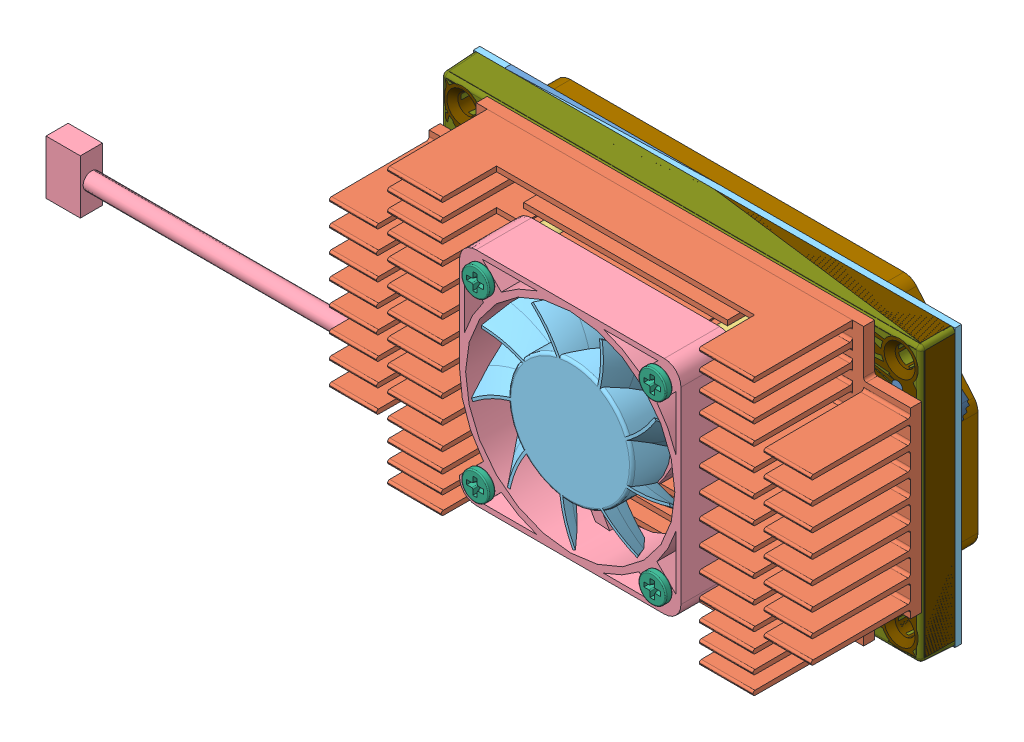
SolidWorks assembly JETSON-NEW_ASM, configuration Default. Lengths in mm.
Overall size (144.7 50.01 33.46).
1881 component instances, 227 part files, 0 mates.
Components (placement in the parent):
- 244-82180-1000-A01-07-31-15_ASM-1: 244-82180-1000-A01-07-31-15_ASM [Default] at origin size (87 50 8.3)
  - 142-82180-1000-A01-07-31-15-1: 142-82180-1000-A01-07-31-15 [Default] at origin size (87 50 1.16)
  - 316-0254-000_2-1: 316-0254-000_2 [Default] at (68.553 22.011 0) x (1 0 0) z (0 0 -1) size (3.51 3.51 0.8)
  - 316-0254-000_2-2: 316-0254-000_2 [Default] at (58.553 17.504 0) x (0 1 0) z (0 0 -1) size (3.51 3.51 0.8)
  - 032-0637-000_1-1: 032-0637-000_1 [Default] at (72.8 30 1.164) size (3.82 1.6 1.8)
  - 032-0637-000_1-2: 032-0637-000_1 [Default] at (72.8 32.06 1.164) size (3.82 1.6 1.8)
  - 032-0628-000_1-1: 032-0628-000_1 [Default] at (53.83 22.43 0) x (0 -1 0) z (0 0 -1) size (3.82 1.6 1.8)
  - 032-0628-000_1-2: 032-0628-000_1 [Default] at (55.94 22.44 0) x (0 -1 0) z (0 0 -1) size (3.82 1.6 1.8)
  - 032-0628-000_1-3: 032-0628-000_1 [Default] at (11.83 6.48 1.164) x (0 1 0) z (0 0 1) size (3.82 1.6 1.8)
  - 032-0628-000_1-4: 032-0628-000_1 [Default] at (13.96 6.5 1.164) x (0 1 0) z (0 0 1) size (3.82 1.6 1.8)
  - RES_04_SMD_015X032_0750-1: RES_04_SMD_015X032_0750 [Default] at (12.96 1.05 1.164) x (0 -1 0) z (0 0 1) size (2.76 3.51 0.75)
  - QFN048Q_P040_0060_T045X04_1000-1: QFN048Q_P040_0060_T045X04_1000 [Default] at (74.15 8.8 1.164) x (0 1 0) z (0 0 1) size (6 6 1)
  - 320-1075-000_1-1: 320-1075-000_1 [Default] at (5.85 26.7 1.164) x (-1 0 0) z (0 0 1) size (4.5 0.8 0.86)
  - 320-1075-000_1-2: 320-1075-000_1 [Default] at (16.1 38.75 1.164) size (4.5 0.8 0.86)
  - 320-1075-000_1-3: 320-1075-000_1 [Default] at (20.1 32.7 1.164) x (0 1 0) z (0 0 1) size (4.5 0.8 0.86)
  - 320-1075-000_1-4: 320-1075-000_1 [Default] at (16.1 26.7 1.164) x (-1 0 0) z (0 0 1) size (4.5 0.8 0.86)
  - 320-1075-000_1-5: 320-1075-000_1 [Default] at (5.85 38.75 1.164) size (4.5 0.8 0.86)
  - 320-1075-000_1-6: 320-1075-000_1 [Default] at (1.45 33.95 1.164) x (0 1 0) z (0 0 1) size (4.5 0.8 0.86)
  - 101-0104-000_2-1: 101-0104-000_2 [Default] at (3.212 36.749 1.164) x (0 1 0) z (0 0 1) size (2.02 1.5 1.01)
  - 101-0104-000_2-2: 101-0104-000_2 [Default] at (3.212 31.163 1.164) x (0 1 0) z (0 0 1) size (2.02 1.5 1.01)
  - T210-INT-DSC-A1_1-1: T210-INT-DSC-A1_1 [Default] at (36.553 18.804 1.164) size (16.2 16.2 1)
  - 115-1605-000_1-1: 115-1605-000_1 [Default] at (67.968 40.894 0) x (0 -1 0) z (0 0 -1) size (2.51 2.01 0.41)
  - 080-1277-000_4-P180-1: 080-1277-000_4-P180 [Default] at (39.5 3.4 0) x (1 0 0) z (0 0 -1) size (70.45 12.44 1)
  - 041-0210-000_1-1: 041-0210-000_1 [Default] at (49.2 15.086 1.164) x (0 -1 0) z (0 0 1) size (8.63 4.4 1.22)
  - 041-0210-000_1-2: 041-0210-000_1 [Default] at (54.05 33.296 0) x (1 0 0) z (0 0 -1) size (8.63 4.4 1.22)
  - 041-0210-000_1-3: 041-0210-000_1 [Default] at (49.99 14.669 0) x (1 0 0) z (0 0 -1) size (8.63 4.4 1.22)
  - 041-0210-000_1-4: 041-0210-000_1 [Default] at (58.51 28.426 0) x (1 0 0) z (0 0 -1) size (8.63 4.4 1.22)
  - 115-1265-000_1-1: 115-1265-000_1 [Default] at (25.202 12.934 0) x (-1 0 0) z (0 0 -1) size (0.96 0.96 0.33)
  - 115-1265-000_1-2: 115-1265-000_1 [Default] at (24.482 16.764 0) x (-1 0 0) z (0 0 -1) size (0.96 0.96 0.33)
  - 316-0420-000_3-1: 316-0420-000_3 [Default] at (6.32 10.69 1.164) size (3.5 3.5 1)
  - 316-0420-000_3-2: 316-0420-000_3 [Default] at (73.91 35.696 1.164) x (0 -1 0) z (0 0 1) size (3.5 3.5 1)
  - 130-0693-000_1-1: 130-0693-000_1 [Default] at (67.584 34.59 1.164) x (0 -1 0) z (0 0 1) size (6.2 4.9 1.8)
  - 130-0692-000_1-1: 130-0692-000_1 [Default] at (7.39 4.464 1.164) size (6.2 4.9 1.8)
  - 115-1066-000_2-1: 115-1066-000_2 [Default] at (72.703 34.834 0) x (1 0 0) z (0 0 -1) size (4.59 4.59 1)
  - 115-1272-000_1-1: 115-1272-000_1 [Default] at (19.03 31.279 0) x (0 1 0) z (0 0 -1) size (0.76 0.76 0.39)
  - 115-1272-000_1-2: 115-1272-000_1 [Default] at (14.95 40.6 0) x (0 1 0) z (0 0 -1) size (0.76 0.76 0.39)
  - 115-1156-000_1-1: 115-1156-000_1 [Default] at (49.173 28.444 0) x (0 -1 0) z (0 0 -1) size (2 2.5 0.8)
  - 115-1659-000_1-1: 115-1659-000_1 [Default] at (15.353 33.154 1.164) x (0 -1 0) z (0 0 1) size (4.87 7.71 0.31)
  - 115-1264-000_1-1: 115-1264-000_1 [Default] at (5.393 34.434 1.164) x (-1 0 0) z (0 0 1) size (1.2 1.2 0.51)
  - 115-1264-000_1-2: 115-1264-000_1 [Default] at (8.309 31.804 1.164) x (-1 0 0) z (0 0 1) size (1.2 1.2 0.51)
  - 115-1264-000_1-3: 115-1264-000_1 [Default] at (7.013 29.684 1.164) x (-1 0 0) z (0 0 1) size (1.2 1.2 0.51)
  - 115-1263-000_1-1: 115-1263-000_1 [Default] at (8.897 36.999 1.164) size (2.01 1.5 0.5)
  - 315-0931-000_1-1: 315-0931-000_1 [Default] at (58.803 35.664 1.164) size (4.08 3.78 0.45)
  - 115-0880-000_1-1: 115-0880-000_1 [Default] at (48.278 39.304 0) x (1 0 0) z (0 0 -1) size (3 5.85 1.1)
  - 170-0212-000_2-1: 170-0212-000_2 [Default] at (10.6 18.8 1.164) x (0 -1 0) z (0 0 1) size (11.5 13 0.48)
  - 174-0133-000_1-1: 174-0133-000_1 [Default] at (18.058 40.074 0) x (1 0 0) z (0 0 -1) size (2 3.52 0.55)
  - 215-0249-000_1-1: 215-0249-000_1 [Default] at (59.32 33.436 0) x (0 1 0) z (0 0 -1) size (2.2 1 0.7)
  - 085-0174-000_1-1: 085-0174-000_1 [Default] at (61.96 37.206 1.164) x (0 1 0) z (0 0 1) size (2.2 1.4 0.6)
  - 130-0293-000_1-1: 130-0293-000_1 [Default] at (-1.8 31.15 1.164) x (-1 0 0) z (0 0 1) size (0.69 0.32 0.36)
  - 130-0293-000_1-2: 130-0293-000_1 [Default] at (-1.75 36.75 1.164) x (-1 0 0) z (0 0 1) size (0.69 0.32 0.36)
  - 130-0293-000_1-3: 130-0293-000_1 [Default] at (9.894 30.222 1.164) x (-1 0 0) z (0 0 1) size (0.69 0.32 0.36)
  - 032-0640-000_1-1: 032-0640-000_1 [Default] at (10.709 29.981 1.164) x (0 -1 0) z (0 0 1) size (0.69 0.32 0.34)
  - 195-2117-000_1-1: 195-2117-000_1 [Default] at (67.3 11.45 0) x (-1 0 0) z (0 0 -1) size (0.69 0.32 0.31)
  - 195-1636-000_1-1: 195-1636-000_1 [Default] at (68.5 29.95 0) x (-1 0 0) z (0 0 -1) size (0.69 0.32 0.31)
  - 195-1636-000_1-2: 195-1636-000_1 [Default] at (10.2 12.1 0) x (0 -1 0) z (0 0 -1) size (0.69 0.32 0.31)
  - 039-0120-000_1-1: 039-0120-000_1 [Default] at (71.15 26.95 0) x (0 1 0) z (0 0 -1) size (0.69 0.32 0.34)
  - 195-2006-000_1-1: 195-2006-000_1 [Default] at (19.3 24.5 0) x (0 1 0) z (0 0 -1) size (0.69 0.32 0.31)
  - 195-2006-000_1-2: 195-2006-000_1 [Default] at (20.35 21.9 0) x (1 0 0) z (0 0 -1) size (0.69 0.32 0.31)
  - 039-0165-000_1-1: 039-0165-000_1 [Default] at (70.54 37.626 0) x (0 1 0) z (0 0 -1) size (0.69 0.32 0.34)
  - 039-0165-000_1-2: 039-0165-000_1 [Default] at (66.428 40.056 0) x (0 -1 0) z (0 0 -1) size (0.69 0.32 0.34)
  - 195-1636-000_1-3: 195-1636-000_1 [Default] at (69.1 39.206 0) x (0 -1 0) z (0 0 -1) size (0.69 0.32 0.31)
  - 039-0161-000_1-1: 039-0161-000_1 [Default] at (68.56 39.206 0) x (0 -1 0) z (0 0 -1) size (0.69 0.32 0.34)
  - 035-0243-000_2-1: 035-0243-000_2 [Default] at (19.65 20.85 1.164) x (-1 0 0) z (0 0 1) size (0.69 0.32 0.34)
  - 130-0344-000_1-1: 130-0344-000_1 [Default] at (9.138 34.734 1.164) x (-1 0 0) z (0 0 1) size (0.69 0.32 0.34)
  - 195-1636-000_1-4: 195-1636-000_1 [Default] at (75.45 36.836 0) x (0 -1 0) z (0 0 -1) size (0.69 0.32 0.31)
  - 195-2034-000_1-1: 195-2034-000_1 [Default] at (30.5 10.1 1.164) x (0 -1 0) z (0 0 1) size (0.69 0.32 0.31)
  - 195-2034-000_1-2: 195-2034-000_1 [Default] at (47.3 23.95 1.164) size (0.69 0.32 0.31)
  - 195-1636-000_1-5: 195-1636-000_1 [Default] at (75.453 35.934 0) x (0 1 0) z (0 0 -1) size (0.69 0.32 0.31)
  - 195-1636-000_1-6: 195-1636-000_1 [Default] at (75.453 35.034 0) x (0 -1 0) z (0 0 -1) size (0.69 0.32 0.31)
  - 195-2002-000_1-1: 195-2002-000_1 [Default] at (77.75 33.95 0) x (1 0 0) z (0 0 -1) size (0.69 0.32 0.31)
  - 195-2002-000_1-2: 195-2002-000_1 [Default] at (74.5 30.85 0) x (1 0 0) z (0 0 -1) size (0.69 0.32 0.31)
  - 195-2002-000_1-3: 195-2002-000_1 [Default] at (68.7 33.75 0) x (1 0 0) z (0 0 -1) size (0.69 0.32 0.31)
  - 195-2118-000_1-1: 195-2118-000_1 [Default] at (58.9 8 1.164) x (0 -1 0) z (0 0 1) size (0.69 0.32 0.31)
  - 195-2118-000_1-2: 195-2118-000_1 [Default] at (57.55 8.25 1.164) x (-1 0 0) z (0 0 1) size (0.69 0.32 0.31)
  - 195-2118-000_1-3: 195-2118-000_1 [Default] at (58.3 8 1.164) x (0 -1 0) z (0 0 1) size (0.69 0.32 0.31)
  - 195-2005-000_1-1: 195-2005-000_1 [Default] at (16.46 40.946 0) x (-1 0 0) z (0 0 -1) size (0.69 0.32 0.31)
  - 195-2005-000_1-2: 195-2005-000_1 [Default] at (16.46 41.476 0) x (1 0 0) z (0 0 -1) size (0.69 0.32 0.31)
  - 195-2005-000_1-3: 195-2005-000_1 [Default] at (17.26 42.436 0) x (0 1 0) z (0 0 -1) size (0.69 0.32 0.31)
  - 195-2005-000_1-4: 195-2005-000_1 [Default] at (17.79 42.436 0) x (0 -1 0) z (0 0 -1) size (0.69 0.32 0.31)
  - 195-2005-000_1-5: 195-2005-000_1 [Default] at (18.85 42.436 0) x (0 1 0) z (0 0 -1) size (0.69 0.32 0.31)
  - 195-2005-000_1-6: 195-2005-000_1 [Default] at (18.32 42.436 0) x (0 -1 0) z (0 0 -1) size (0.69 0.32 0.31)
  - 195-1636-000_1-7: 195-1636-000_1 [Default] at (77.91 33.886 1.164) x (-1 0 0) z (0 0 1) size (0.69 0.32 0.31)
  - 195-1636-000_1-8: 195-1636-000_1 [Default] at (0.59 16.124 1.164) size (0.69 0.32 0.31)
  - 039-0165-000_1-3: 039-0165-000_1 [Default] at (51.7 9.8 1.164) x (0 1 0) z (0 0 1) size (0.69 0.32 0.34)
  - 195-2005-000_1-7: 195-2005-000_1 [Default] at (52.3 9.8 1.164) x (0 -1 0) z (0 0 1) size (0.69 0.32 0.31)
  - 195-1636-000_1-9: 195-1636-000_1 [Default] at (18.556 17.72 0) x (1 0 0) z (0 0 -1) size (0.69 0.32 0.31)
  - 195-1636-000_1-10: 195-1636-000_1 [Default] at (18.556 18.25 0) x (1 0 0) z (0 0 -1) size (0.69 0.32 0.31)
  - 195-1636-000_1-11: 195-1636-000_1 [Default] at (18.556 16.03 0) x (1 0 0) z (0 0 -1) size (0.69 0.32 0.31)
  - 195-1636-000_1-12: 195-1636-000_1 [Default] at (18.556 16.56 0) x (1 0 0) z (0 0 -1) size (0.69 0.32 0.31)
  - 195-1636-000_1-13: 195-1636-000_1 [Default] at (18.076 17.72 0) x (-1 0 0) z (0 0 -1) size (0.69 0.32 0.31)
  - 195-1636-000_1-14: 195-1636-000_1 [Default] at (18.076 18.25 0) x (-1 0 0) z (0 0 -1) size (0.69 0.32 0.31)
  - 195-1636-000_1-15: 195-1636-000_1 [Default] at (18.076 16.03 0) x (-1 0 0) z (0 0 -1) size (0.69 0.32 0.31)
  - 195-1636-000_1-16: 195-1636-000_1 [Default] at (18.076 16.56 0) x (-1 0 0) z (0 0 -1) size (0.69 0.32 0.31)
  - 035-0243-000_2-2: 035-0243-000_2 [Default] at (46.54 8.126 1.164) size (0.69 0.32 0.34)
  - 195-1636-000_1-17: 195-1636-000_1 [Default] at (47.72 10.92 0) x (0 -1 0) z (0 0 -1) size (0.69 0.32 0.31)
  - 195-2006-000_1-3: 195-2006-000_1 [Default] at (27.25 11.55 0) x (0 -1 0) z (0 0 -1) size (0.69 0.32 0.31)
  - 195-2006-000_1-4: 195-2006-000_1 [Default] at (26.7 11.55 0) x (0 -1 0) z (0 0 -1) size (0.69 0.32 0.31)
  - 130-0298-000_1-1: 130-0298-000_1 [Default] at (9.06 29.981 1.164) x (0 -1 0) z (0 0 1) size (0.69 0.32 0.36)
  - 195-1636-000_1-18: 195-1636-000_1 [Default] at (37.032 14.474 0) x (0 1 0) z (0 0 -1) size (0.69 0.32 0.31)
  - 039-0165-000_1-4: 039-0165-000_1 [Default] at (24.013 41.3 0) x (0 -1 0) z (0 0 -1) size (0.69 0.32 0.34)
  - 195-2117-000_1-2: 195-2117-000_1 [Default] at (17.2 22.6 0) x (-1 0 0) z (0 0 -1) size (0.69 0.32 0.31)
  - 195-2006-000_1-5: 195-2006-000_1 [Default] at (11.65 13.25 0) x (1 0 0) z (0 0 -1) size (0.69 0.32 0.31)
  - 039-0165-000_1-5: 039-0165-000_1 [Default] at (25.333 34.244 0) x (-1 0 0) z (0 0 -1) size (0.69 0.32 0.34)
  - 039-0165-000_1-6: 039-0165-000_1 [Default] at (24.953 34.944 0) x (-1 0 0) z (0 0 -1) size (0.69 0.32 0.34)
  - 195-2117-000_1-3: 195-2117-000_1 [Default] at (7.6 20.05 0) x (1 0 0) z (0 0 -1) size (0.69 0.32 0.31)
  - 195-2117-000_1-4: 195-2117-000_1 [Default] at (18.65 11.7 0) x (0 -1 0) z (0 0 -1) size (0.69 0.32 0.31)
  - 039-0165-000_1-7: 039-0165-000_1 [Default] at (22.7 38.65 0) x (0 1 0) z (0 0 -1) size (0.69 0.32 0.34)
  - 039-0165-000_1-8: 039-0165-000_1 [Default] at (23.453 38.834 0) x (-1 0 0) z (0 0 -1) size (0.69 0.32 0.34)
  - 039-0165-000_1-9: 039-0165-000_1 [Default] at (21.88 39.19 0) x (-1 0 0) z (0 0 -1) size (0.69 0.32 0.34)
  - 195-1758-000_1-1: 195-1758-000_1 [Default] at (21.853 38.444 0) x (-1 0 0) z (0 0 -1) size (0.69 0.32 0.27)
  - 195-1758-000_1-2: 195-1758-000_1 [Default] at (21.823 37.774 0) x (-1 0 0) z (0 0 -1) size (0.69 0.32 0.27)
  - 039-0165-000_1-10: 039-0165-000_1 [Default] at (30.15 32.8 0) x (1 0 0) z (0 0 -1) size (0.69 0.32 0.34)
  - 195-2506-000_1-1: 195-2506-000_1 [Default] at (27.573 24.364 1.164) x (-1 0 0) z (0 0 1) size (0.69 0.32 0.31)
  - 195-2506-000_1-2: 195-2506-000_1 [Default] at (27.7 23.3 1.164) x (-1 0 0) z (0 0 1) size (0.69 0.32 0.31)
  - 039-0165-000_1-11: 039-0165-000_1 [Default] at (25.553 36.004 0) x (1 0 0) z (0 0 -1) size (0.69 0.32 0.34)
  - 039-0165-000_1-12: 039-0165-000_1 [Default] at (26.9 36 0) x (1 0 0) z (0 0 -1) size (0.69 0.32 0.34)
  - 195-2117-000_1-5: 195-2117-000_1 [Default] at (17.2 23.7 0) x (-1 0 0) z (0 0 -1) size (0.69 0.32 0.31)
  - 039-0165-000_1-13: 039-0165-000_1 [Default] at (25.853 32.304 0) x (-1 0 0) z (0 0 -1) size (0.69 0.32 0.34)
  - 035-0243-000_2-3: 035-0243-000_2 [Default] at (25.603 25.814 1.164) x (0 1 0) z (0 0 1) size (0.69 0.32 0.34)
  - 195-1636-000_1-19: 195-1636-000_1 [Default] at (30.95 27.25 0) x (0 1 0) z (0 0 -1) size (0.69 0.32 0.31)
  - 039-0165-000_1-14: 039-0165-000_1 [Default] at (31.368 23.724 0) x (-1 0 0) z (0 0 -1) size (0.69 0.32 0.34)
  - 039-0165-000_1-15: 039-0165-000_1 [Default] at (30.473 23.719 0) x (-1 0 0) z (0 0 -1) size (0.69 0.32 0.34)
  - 195-2117-000_1-6: 195-2117-000_1 [Default] at (30.515 23.194 0) x (1 0 0) z (0 0 -1) size (0.69 0.32 0.31)
  - 039-0165-000_1-16: 039-0165-000_1 [Default] at (31.401 23.194 0) x (-1 0 0) z (0 0 -1) size (0.69 0.32 0.34)
  - 195-1636-000_1-20: 195-1636-000_1 [Default] at (67.75 12.2 0) x (0 -1 0) z (0 0 -1) size (0.69 0.32 0.31)
  - 039-0165-000_1-17: 039-0165-000_1 [Default] at (32.1 33 0) x (-1 0 0) z (0 0 -1) size (0.69 0.32 0.34)
  - 039-0165-000_1-18: 039-0165-000_1 [Default] at (33.713 34.804 0) x (0 1 0) z (0 0 -1) size (0.69 0.32 0.34)
  - 039-0165-000_1-19: 039-0165-000_1 [Default] at (32.583 23.814 0) x (-1 0 0) z (0 0 -1) size (0.69 0.32 0.34)
  - 039-0165-000_1-20: 039-0165-000_1 [Default] at (32.323 23.294 0) x (1 0 0) z (0 0 -1) size (0.69 0.32 0.34)
  - 195-1636-000_1-21: 195-1636-000_1 [Default] at (37.4 29.65 0) x (-1 0 0) z (0 0 -1) size (0.69 0.32 0.31)
  - 039-0165-000_1-21: 039-0165-000_1 [Default] at (11.65 14.4 0) x (1 0 0) z (0 0 -1) size (0.69 0.32 0.34)
  - 195-2006-000_1-6: 195-2006-000_1 [Default] at (11.65 13.85 0) x (1 0 0) z (0 0 -1) size (0.69 0.32 0.31)
  - 039-0165-000_1-22: 039-0165-000_1 [Default] at (32.5 41.35 0) x (0 -1 0) z (0 0 -1) size (0.69 0.32 0.34)
  - 039-0165-000_1-23: 039-0165-000_1 [Default] at (35.733 34.964 0) x (0 -1 0) z (0 0 -1) size (0.69 0.32 0.34)
  - 195-2005-000_1-8: 195-2005-000_1 [Default] at (32.265 27.36 0) x (-1 0 0) z (0 0 -1) size (0.69 0.32 0.31)
  - 195-1636-000_1-22: 195-1636-000_1 [Default] at (35.358 25.641 0) x (1 0 0) z (0 0 -1) size (0.69 0.32 0.31)
  - 039-0165-000_1-24: 039-0165-000_1 [Default] at (36.07 25.804 0) x (0 1 0) z (0 0 -1) size (0.69 0.32 0.34)
  - 039-0165-000_1-25: 039-0165-000_1 [Default] at (39.603 39.284 0) x (0 1 0) z (0 0 -1) size (0.69 0.32 0.34)
  - 039-0165-000_1-26: 039-0165-000_1 [Default] at (39.733 34.784 0) x (-1 0 0) z (0 0 -1) size (0.69 0.32 0.34)
  - 039-0165-000_1-27: 039-0165-000_1 [Default] at (40.473 23.854 0) x (0 1 0) z (0 0 -1) size (0.69 0.32 0.34)
  - 039-0165-000_1-28: 039-0165-000_1 [Default] at (37.453 39.204 0) x (-1 0 0) z (0 0 -1) size (0.69 0.32 0.34)
  - 195-1758-000_1-3: 195-1758-000_1 [Default] at (37.75 38.15 0) x (0 -1 0) z (0 0 -1) size (0.69 0.32 0.27)
  - 195-1758-000_1-4: 195-1758-000_1 [Default] at (37.8 35.75 0) x (0 -1 0) z (0 0 -1) size (0.69 0.32 0.27)
  - 039-0165-000_1-29: 039-0165-000_1 [Default] at (38.7 36 0) x (1 0 0) z (0 0 -1) size (0.69 0.32 0.34)
  - 039-0165-000_1-30: 039-0165-000_1 [Default] at (38.7 34.4 0) x (1 0 0) z (0 0 -1) size (0.69 0.32 0.34)
  - 039-0165-000_1-31: 039-0165-000_1 [Default] at (42 32.8 0) x (-1 0 0) z (0 0 -1) size (0.69 0.32 0.34)
  - 039-0165-000_1-32: 039-0165-000_1 [Default] at (39.75 33.05 0) x (0 1 0) z (0 0 -1) size (0.69 0.32 0.34)
  - 195-2005-000_1-9: 195-2005-000_1 [Default] at (40.728 29.454 0) x (0 -1 0) z (0 0 -1) size (0.69 0.32 0.31)
  - 195-1636-000_1-23: 195-1636-000_1 [Default] at (40.853 28.394 0) x (1 0 0) z (0 0 -1) size (0.69 0.32 0.31)
  - 039-0165-000_1-33: 039-0165-000_1 [Default] at (41.752 23.379 0) x (0 1 0) z (0 0 -1) size (0.69 0.32 0.34)
  - 195-2005-000_1-10: 195-2005-000_1 [Default] at (42.903 40.854 0) x (-1 0 0) z (0 0 -1) size (0.69 0.32 0.31)
  - 195-2006-000_1-7: 195-2006-000_1 [Default] at (42.753 39.054 0) x (0 -1 0) z (0 0 -1) size (0.69 0.32 0.31)
  - 195-2006-000_1-8: 195-2006-000_1 [Default] at (42.763 39.967 0) x (0 1 0) z (0 0 -1) size (0.69 0.32 0.31)
  - 039-0165-000_1-34: 039-0165-000_1 [Default] at (44.25 39.95 0) x (1 0 0) z (0 0 -1) size (0.69 0.32 0.34)
  - 039-0165-000_1-35: 039-0165-000_1 [Default] at (42.753 38.054 0) x (0 -1 0) z (0 0 -1) size (0.69 0.32 0.34)
  - 195-1636-000_1-24: 195-1636-000_1 [Default] at (42.9 35.2 0) x (0 -1 0) z (0 0 -1) size (0.69 0.32 0.31)
  - 039-0165-000_1-36: 039-0165-000_1 [Default] at (43.65 35.2 0) x (0 -1 0) z (0 0 -1) size (0.69 0.32 0.34)
  - 195-1636-000_1-25: 195-1636-000_1 [Default] at (41.4 34.05 0) x (1 0 0) z (0 0 -1) size (0.69 0.32 0.31)
  - 039-0165-000_1-37: 039-0165-000_1 [Default] at (43.7 34.15 0) x (0 -1 0) z (0 0 -1) size (0.69 0.32 0.34)
  - 039-0165-000_1-38: 039-0165-000_1 [Default] at (47.623 34.054 0) x (-1 0 0) z (0 0 -1) size (0.69 0.32 0.34)
  - 039-0165-000_1-39: 039-0165-000_1 [Default] at (48.447 33.88 0) x (0 -1 0) z (0 0 -1) size (0.69 0.32 0.34)
  - 195-2005-000_1-11: 195-2005-000_1 [Default] at (47.263 26.769 0) x (1 0 0) z (0 0 -1) size (0.69 0.32 0.31)
  - 039-0165-000_1-40: 039-0165-000_1 [Default] at (46.253 38.504 0) x (0 1 0) z (0 0 -1) size (0.69 0.32 0.34)
  - 039-0165-000_1-41: 039-0165-000_1 [Default] at (46.603 37.074 0) x (0 -1 0) z (0 0 -1) size (0.69 0.32 0.34)
  - 195-2002-000_1-4: 195-2002-000_1 [Default] at (46.55 34.9 0) x (1 0 0) z (0 0 -1) size (0.69 0.32 0.31)
  - 039-0165-000_1-42: 039-0165-000_1 [Default] at (47.15 32.9 0) x (1 0 0) z (0 0 -1) size (0.69 0.32 0.34)
  - 039-0165-000_1-43: 039-0165-000_1 [Default] at (44.25 38.9 0) x (1 0 0) z (0 0 -1) size (0.69 0.32 0.34)
  - 039-0165-000_1-44: 039-0165-000_1 [Default] at (43.853 36.604 0) x (-1 0 0) z (0 0 -1) size (0.69 0.32 0.34)
  - 039-0165-000_1-45: 039-0165-000_1 [Default] at (45.353 34.444 0) x (-1 0 0) z (0 0 -1) size (0.69 0.32 0.34)
  - 039-0165-000_1-46: 039-0165-000_1 [Default] at (45.5 32.55 0) x (0 -1 0) z (0 0 -1) size (0.69 0.32 0.34)
  - 039-0165-000_1-47: 039-0165-000_1 [Default] at (43.65 33.05 0) x (0 1 0) z (0 0 -1) size (0.69 0.32 0.34)
  - 195-1636-000_1-26: 195-1636-000_1 [Default] at (48.94 10.93 0) x (0 -1 0) z (0 0 -1) size (0.69 0.32 0.31)
  - 039-0165-000_1-48: 039-0165-000_1 [Default] at (50.928 40.754 0) x (1 0 0) z (0 0 -1) size (0.69 0.32 0.34)
  - 039-0165-000_1-49: 039-0165-000_1 [Default] at (49.163 33.855 0) x (0 -1 0) z (0 0 -1) size (0.69 0.32 0.34)
  - 039-0165-000_1-50: 039-0165-000_1 [Default] at (51.243 29.284 0) x (1 0 0) z (0 0 -1) size (0.69 0.32 0.34)
  - 039-0165-000_1-51: 039-0165-000_1 [Default] at (50.503 39.654 0) x (-1 0 0) z (0 0 -1) size (0.69 0.32 0.34)
  - 039-0165-000_1-52: 039-0165-000_1 [Default] at (50.503 38.954 0) x (-1 0 0) z (0 0 -1) size (0.69 0.32 0.34)
  - 039-0165-000_1-53: 039-0165-000_1 [Default] at (49.853 36.179 0) x (0 1 0) z (0 0 -1) size (0.69 0.32 0.34)
  - 039-0165-000_1-54: 039-0165-000_1 [Default] at (50.314 37.05 0) x (-1 0 0) z (0 0 -1) size (0.69 0.32 0.34)
  - 195-2002-000_1-5: 195-2002-000_1 [Default] at (47.45 34.9 0) x (-1 0 0) z (0 0 -1) size (0.69 0.32 0.31)
  - 039-0165-000_1-55: 039-0165-000_1 [Default] at (48.879 32.877 0) x (-1 0 0) z (0 0 -1) size (0.69 0.32 0.34)
  - 195-1636-000_1-27: 195-1636-000_1 [Default] at (48.34 10.93 0) x (0 -1 0) z (0 0 -1) size (0.69 0.32 0.31)
  - 035-0122-000_1-1: 035-0122-000_1 [Default] at (4.828 35.604 1.164) x (0 1 0) z (0 0 1) size (0.69 0.32 0.34)
  - 195-1636-000_1-28: 195-1636-000_1 [Default] at (4.753 32.979 1.164) x (-1 0 0) z (0 0 1) size (0.69 0.32 0.31)
  - 195-1636-000_1-29: 195-1636-000_1 [Default] at (4.512 32.738 1.164) x (0 1 0) z (0 0 1) size (0.69 0.32 0.31)
  - 035-0122-000_1-2: 035-0122-000_1 [Default] at (4.078 33.854 1.164) x (-1 0 0) z (0 0 1) size (0.69 0.32 0.34)
  - 195-1636-000_1-30: 195-1636-000_1 [Default] at (5.061 30.945 1.164) x (-1 0 0) z (0 0 1) size (0.69 0.32 0.31)
  - 130-0330-000_1-1: 130-0330-000_1 [Default] at (4.408 29.445 1.164) x (0 -1 0) z (0 0 1) size (0.69 0.32 0.34)
  - 035-0243-000_2-4: 035-0243-000_2 [Default] at (5.191 29.686 1.164) x (-1 0 0) z (0 0 1) size (0.69 0.32 0.34)
  - 195-2005-000_1-12: 195-2005-000_1 [Default] at (5.423 27.972 1.164) x (0 -1 0) z (0 0 1) size (0.69 0.32 0.31)
  - 195-2005-000_1-13: 195-2005-000_1 [Default] at (4.705 27.972 1.164) x (0 -1 0) z (0 0 1) size (0.69 0.32 0.31)
  - 039-0165-000_1-56: 039-0165-000_1 [Default] at (18.95 30.45 0) x (-1 0 0) z (0 0 -1) size (0.69 0.32 0.34)
  - 130-0330-000_1-2: 130-0330-000_1 [Default] at (3.596 35.184 1.164) x (-1 0 0) z (0 0 1) size (0.69 0.32 0.34)
  - 035-0243-000_2-5: 035-0243-000_2 [Default] at (3.503 32.979 1.164) x (-1 0 0) z (0 0 1) size (0.69 0.32 0.34)
  - 195-1636-000_1-31: 195-1636-000_1 [Default] at (4.533 25.324 1.164) x (0 1 0) z (0 0 1) size (0.69 0.32 0.31)
  - 035-0243-000_2-6: 035-0243-000_2 [Default] at (8.235 29.188 1.164) x (-1 0 0) z (0 0 1) size (0.69 0.32 0.34)
  - 195-2005-000_1-14: 195-2005-000_1 [Default] at (8.218 25.314 1.164) x (0 -1 0) z (0 0 1) size (0.69 0.32 0.31)
  - 195-1636-000_1-32: 195-1636-000_1 [Default] at (7.7 25.314 1.164) x (0 1 0) z (0 0 1) size (0.69 0.32 0.31)
  - 195-1636-000_1-33: 195-1636-000_1 [Default] at (8.736 25.314 1.164) x (0 1 0) z (0 0 1) size (0.69 0.32 0.31)
  - 195-1636-000_1-34: 195-1636-000_1 [Default] at (5.814 36.455 1.164) x (-1 0 0) z (0 0 1) size (0.69 0.32 0.31)
  - 035-0243-000_2-7: 035-0243-000_2 [Default] at (6.599 34.734 1.164) x (-1 0 0) z (0 0 1) size (0.69 0.32 0.34)
  - 035-0243-000_2-8: 035-0243-000_2 [Default] at (5.823 35.854 1.164) x (-1 0 0) z (0 0 1) size (0.69 0.32 0.34)
  - 195-1636-000_1-35: 195-1636-000_1 [Default] at (6.723 35.854 1.164) x (-1 0 0) z (0 0 1) size (0.69 0.32 0.31)
  - 035-0243-000_2-9: 035-0243-000_2 [Default] at (6.599 33.749 1.164) x (-1 0 0) z (0 0 1) size (0.69 0.32 0.34)
  - 035-0243-000_2-10: 035-0243-000_2 [Default] at (6.51 31.341 1.164) size (0.69 0.32 0.34)
  - 035-0243-000_2-11: 035-0243-000_2 [Default] at (6.787 32.049 1.164) x (0 -1 0) z (0 0 1) size (0.69 0.32 0.34)
  - 195-1636-000_1-36: 195-1636-000_1 [Default] at (6.269 32.049 1.164) x (0 -1 0) z (0 0 1) size (0.69 0.32 0.31)
  - 035-0122-000_1-3: 035-0122-000_1 [Default] at (5.803 30.204 1.164) x (-1 0 0) z (0 0 1) size (0.69 0.32 0.34)
  - 035-0122-000_1-4: 035-0122-000_1 [Default] at (5.703 29.004 1.164) x (-1 0 0) z (0 0 1) size (0.69 0.32 0.34)
  - 195-2005-000_1-15: 195-2005-000_1 [Default] at (6.108 27.972 1.164) x (0 -1 0) z (0 0 1) size (0.69 0.32 0.31)
  - 039-0165-000_1-57: 039-0165-000_1 [Default] at (9.35 17.8 0) x (0 -1 0) z (0 0 -1) size (0.69 0.32 0.34)
  - 195-1636-000_1-37: 195-1636-000_1 [Default] at (6.146 25.314 1.164) x (0 1 0) z (0 0 1) size (0.69 0.32 0.31)
  - 195-1636-000_1-38: 195-1636-000_1 [Default] at (6.664 25.314 1.164) x (0 1 0) z (0 0 1) size (0.69 0.32 0.31)
  - 195-1636-000_1-39: 195-1636-000_1 [Default] at (7.182 25.314 1.164) x (0 1 0) z (0 0 1) size (0.69 0.32 0.31)
  - 195-1636-000_1-40: 195-1636-000_1 [Default] at (5.628 25.314 1.164) x (0 1 0) z (0 0 1) size (0.69 0.32 0.31)
  - 195-2006-000_1-9: 195-2006-000_1 [Default] at (17.687 31.24 0) x (0 -1 0) z (0 0 -1) size (0.69 0.32 0.31)
  - 195-1636-000_1-41: 195-1636-000_1 [Default] at (5.103 37.229 1.164) x (0 -1 0) z (0 0 1) size (0.69 0.32 0.31)
  - 035-0243-000_2-12: 035-0243-000_2 [Default] at (4.55 36.747 1.164) x (0 -1 0) z (0 0 1) size (0.69 0.32 0.34)
  - 195-1636-000_1-42: 195-1636-000_1 [Default] at (5.103 36.747 1.164) x (0 1 0) z (0 0 1) size (0.69 0.32 0.31)
  - 035-0243-000_2-13: 035-0243-000_2 [Default] at (4.078 34.434 1.164) x (-1 0 0) z (0 0 1) size (0.69 0.32 0.34)
  - 130-0334-000_1-1: 130-0334-000_1 [Default] at (9.408 35.498 1.164) x (0 -1 0) z (0 0 1) size (0.69 0.32 0.34)
  - 035-0105-000_1-1: 035-0105-000_1 [Default] at (10.11 35.738 1.164) size (0.69 0.32 0.34)
  - 130-0280-000_1-1: 130-0280-000_1 [Default] at (9.959 34.495 1.164) x (0 -1 0) z (0 0 1) size (0.69 0.32 0.36)
  - 035-0105-000_1-2: 035-0105-000_1 [Default] at (8.706 35.739 1.164) size (0.69 0.32 0.34)
  - 130-0330-000_1-3: 130-0330-000_1 [Default] at (9.78 32.603 1.164) x (0 -1 0) z (0 0 1) size (0.69 0.32 0.34)
  - 035-0243-000_2-14: 035-0243-000_2 [Default] at (10.088 33.749 1.164) x (-1 0 0) z (0 0 1) size (0.69 0.32 0.34)
  - 130-0330-000_1-4: 130-0330-000_1 [Default] at (9.381 33.989 1.164) x (0 1 0) z (0 0 1) size (0.69 0.32 0.34)
  - 035-0105-000_1-3: 035-0105-000_1 [Default] at (9.009 32.844 1.164) size (0.69 0.32 0.34)
  - 035-0105-000_1-4: 035-0105-000_1 [Default] at (10.39 32.142 1.164) x (0 1 0) z (0 0 1) size (0.69 0.32 0.34)
  - 130-0334-000_1-2: 130-0334-000_1 [Default] at (9.861 31.66 1.164) x (0 -1 0) z (0 0 1) size (0.69 0.32 0.34)
  - 035-0105-000_1-5: 035-0105-000_1 [Default] at (9.343 31.66 1.164) x (0 1 0) z (0 0 1) size (0.69 0.32 0.34)
  - 130-0330-000_1-5: 130-0330-000_1 [Default] at (9.602 29.429 1.164) x (0 1 0) z (0 0 1) size (0.69 0.32 0.34)
  - 195-2005-000_1-16: 195-2005-000_1 [Default] at (10.223 27.779 1.164) size (0.69 0.32 0.31)
  - 195-1636-000_1-43: 195-1636-000_1 [Default] at (9.254 25.314 1.164) x (0 1 0) z (0 0 1) size (0.69 0.32 0.31)
  - 035-0122-000_1-5: 035-0122-000_1 [Default] at (7.483 37.064 1.164) x (0 -1 0) z (0 0 1) size (0.69 0.32 0.34)
  - 035-0243-000_2-15: 035-0243-000_2 [Default] at (7.483 35.613 1.164) x (0 -1 0) z (0 0 1) size (0.69 0.32 0.34)
  - 130-0298-000_1-2: 130-0298-000_1 [Default] at (8.358 34.495 1.164) x (0 -1 0) z (0 0 1) size (0.69 0.32 0.36)
  - 035-0122-000_1-6: 035-0122-000_1 [Default] at (8.004 35.549 1.164) x (0 -1 0) z (0 0 1) size (0.69 0.32 0.34)
  - 035-0122-000_1-7: 035-0122-000_1 [Default] at (8.043 32.844 1.164) size (0.69 0.32 0.34)
  - 035-0122-000_1-8: 035-0122-000_1 [Default] at (7.235 30.984 1.164) x (0 -1 0) z (0 0 1) size (0.69 0.32 0.34)
  - 035-0122-000_1-9: 035-0122-000_1 [Default] at (7.305 32.049 1.164) x (0 1 0) z (0 0 1) size (0.69 0.32 0.34)
  - 035-0243-000_2-16: 035-0243-000_2 [Default] at (8.235 30.222 1.164) x (-1 0 0) z (0 0 1) size (0.69 0.32 0.34)
  - 035-0122-000_1-10: 035-0122-000_1 [Default] at (10.495 37.647 1.164) size (0.69 0.32 0.34)
  - 035-0122-000_1-11: 035-0122-000_1 [Default] at (10.495 37.129 1.164) size (0.69 0.32 0.34)
  - 035-0105-000_1-6: 035-0105-000_1 [Default] at (10.562 32.844 1.164) size (0.69 0.32 0.34)
  - 039-0165-000_1-58: 039-0165-000_1 [Default] at (11.078 33.679 1.164) x (0 1 0) z (0 0 1) size (0.69 0.32 0.34)
  - 035-0243-000_2-17: 035-0243-000_2 [Default] at (10.523 29.188 1.164) x (-1 0 0) z (0 0 1) size (0.69 0.32 0.34)
  - 195-2337-000_1-1: 195-2337-000_1 [Default] at (14.912 30.106 1.164) x (0 1 0) z (0 0 1) size (0.69 0.32 0.31)
  - 035-0135-000_1-1: 035-0135-000_1 [Default] at (14.93 29.21 1.164) x (0 -1 0) z (0 0 1) size (0.69 0.32 0.34)
  - 195-2005-000_1-17: 195-2005-000_1 [Default] at (13.85 41.55 0) x (0 -1 0) z (0 0 -1) size (0.69 0.32 0.31)
  - 039-0165-000_1-59: 039-0165-000_1 [Default] at (13.85 40.55 0) x (0 -1 0) z (0 0 -1) size (0.69 0.32 0.34)
  - 035-0105-000_1-7: 035-0105-000_1 [Default] at (13.573 36.209 1.164) x (0 -1 0) z (0 0 1) size (0.69 0.32 0.34)
  - 035-0105-000_1-8: 035-0105-000_1 [Default] at (12.753 37.409 1.164) size (0.69 0.32 0.34)
  - 195-1636-000_1-44: 195-1636-000_1 [Default] at (13.621 34.372 0) x (0 1 0) z (0 0 -1) size (0.69 0.32 0.31)
  - 035-0135-000_1-2: 035-0135-000_1 [Default] at (13.038 28.694 1.164) x (-1 0 0) z (0 0 1) size (0.69 0.32 0.34)
  - 035-0122-000_1-12: 035-0122-000_1 [Default] at (14.085 37.68 1.164) x (-1 0 0) z (0 0 1) size (0.69 0.32 0.34)
  - 035-0122-000_1-13: 035-0122-000_1 [Default] at (14.106 36.209 1.164) x (0 1 0) z (0 0 1) size (0.69 0.32 0.34)
  - 130-0330-000_1-6: 130-0330-000_1 [Default] at (13.817 36.938 1.164) size (0.69 0.32 0.34)
  - 035-0122-000_1-14: 035-0122-000_1 [Default] at (15.525 36.204 1.164) x (0 1 0) z (0 0 1) size (0.69 0.32 0.34)
  - 039-0165-000_1-60: 039-0165-000_1 [Default] at (15.007 36.204 1.164) x (0 1 0) z (0 0 1) size (0.69 0.32 0.34)
  - 195-1636-000_1-45: 195-1636-000_1 [Default] at (17.087 17.723 0) x (1 0 0) z (0 0 -1) size (0.69 0.32 0.31)
  - 195-1636-000_1-46: 195-1636-000_1 [Default] at (17.1 16.02 0) x (1 0 0) z (0 0 -1) size (0.69 0.32 0.31)
  - 195-1636-000_1-47: 195-1636-000_1 [Default] at (17.05 16.57 0) x (1 0 0) z (0 0 -1) size (0.69 0.32 0.31)
  - 039-0165-000_1-61: 039-0165-000_1 [Default] at (15.397 32.956 0) x (0 -1 0) z (0 0 -1) size (0.69 0.32 0.34)
  - 039-0165-000_1-62: 039-0165-000_1 [Default] at (16.621 39.105 0) x (0 1 0) z (0 0 -1) size (0.69 0.32 0.34)
  - 195-2005-000_1-18: 195-2005-000_1 [Default] at (16.063 36.204 1.164) x (0 1 0) z (0 0 1) size (0.69 0.32 0.31)
  - 195-1636-000_1-48: 195-1636-000_1 [Default] at (17.087 18.25 0) x (1 0 0) z (0 0 -1) size (0.69 0.32 0.31)
  - 039-0199-000_1-1: 039-0199-000_1 [Default] at (16.451 29.906 1.164) x (0 -1 0) z (0 0 1) size (0.69 0.32 0.36)
  - 195-2117-000_1-7: 195-2117-000_1 [Default] at (19.3 11.7 0) x (0 1 0) z (0 0 -1) size (0.69 0.32 0.31)
  - 195-2117-000_1-8: 195-2117-000_1 [Default] at (18.55 17.19 0) x (1 0 0) z (0 0 -1) size (0.69 0.32 0.31)
  - 195-2005-000_1-19: 195-2005-000_1 [Default] at (18.588 36.204 1.164) x (0 1 0) z (0 0 1) size (0.69 0.32 0.31)
  - 195-1636-000_1-49: 195-1636-000_1 [Default] at (17.853 36.204 1.164) x (0 -1 0) z (0 0 1) size (0.69 0.32 0.31)
  - 195-1636-000_1-50: 195-1636-000_1 [Default] at (18.597 34.602 0) x (0 1 0) z (0 0 -1) size (0.69 0.32 0.31)
  - 195-1636-000_1-51: 195-1636-000_1 [Default] at (18.079 34.602 0) x (0 1 0) z (0 0 -1) size (0.69 0.32 0.31)
  - 195-1636-000_1-52: 195-1636-000_1 [Default] at (17.409 34.602 0) x (0 1 0) z (0 0 -1) size (0.69 0.32 0.31)
  - 195-2172-000_1-1: 195-2172-000_1 [Default] at (27.7 14.4 1.164) x (-1 0 0) z (0 0 1) size (0.69 0.32 0.31)
  - 195-2172-000_1-2: 195-2172-000_1 [Default] at (27.723 12.914 1.164) x (-1 0 0) z (0 0 1) size (0.69 0.32 0.31)
  - 195-2487-000_1-1: 195-2487-000_1 [Default] at (26.123 16.104 0) x (0 1 0) z (0 0 -1) size (0.69 0.32 0.31)
  - 195-2006-000_1-10: 195-2006-000_1 [Default] at (24.965 11.846 0) x (0 -1 0) z (0 0 -1) size (0.69 0.32 0.31)
  - 039-0165-000_1-63: 039-0165-000_1 [Default] at (12.35 19.25 0) x (-1 0 0) z (0 0 -1) size (0.69 0.32 0.34)
  - 039-0165-000_1-64: 039-0165-000_1 [Default] at (7.6 21.05 0) x (1 0 0) z (0 0 -1) size (0.69 0.32 0.34)
  - 035-0243-000_2-18: 035-0243-000_2 [Default] at (27.7 21.95 1.164) size (0.69 0.32 0.34)
  - 195-2506-000_1-3: 195-2506-000_1 [Default] at (27.7 16.9 1.164) x (-1 0 0) z (0 0 1) size (0.69 0.32 0.31)
  - 039-0165-000_1-65: 039-0165-000_1 [Default] at (31.213 15.274 0) x (1 0 0) z (0 0 -1) size (0.69 0.32 0.34)
  - 039-0165-000_1-66: 039-0165-000_1 [Default] at (31.903 14.494 0) x (0 1 0) z (0 0 -1) size (0.69 0.32 0.34)
  - 039-0165-000_1-67: 039-0165-000_1 [Default] at (31.183 14.754 0) x (-1 0 0) z (0 0 -1) size (0.69 0.32 0.34)
  - 039-0165-000_1-68: 039-0165-000_1 [Default] at (31.133 14.234 0) x (-1 0 0) z (0 0 -1) size (0.69 0.32 0.34)
  - 039-0165-000_1-69: 039-0165-000_1 [Default] at (31.713 13.704 0) x (-1 0 0) z (0 0 -1) size (0.69 0.32 0.34)
  - 035-0243-000_2-19: 035-0243-000_2 [Default] at (32.85 8.65 1.164) size (0.69 0.32 0.34)
  - 039-0165-000_1-70: 039-0165-000_1 [Default] at (30.533 21.774 0) x (1 0 0) z (0 0 -1) size (0.69 0.32 0.34)
  - 195-2004-000_1-1: 195-2004-000_1 [Default] at (30.109 20.345 0) x (1 0 0) z (0 0 -1) size (0.69 0.32 0.31)
  - 195-1636-000_1-53: 195-1636-000_1 [Default] at (30.003 19.574 0) x (0 1 0) z (0 0 -1) size (0.69 0.32 0.31)
  - 039-0165-000_1-71: 039-0165-000_1 [Default] at (34.778 14.474 0) x (0 1 0) z (0 0 -1) size (0.69 0.32 0.34)
  - 039-0165-000_1-72: 039-0165-000_1 [Default] at (35.296 14.474 0) x (0 1 0) z (0 0 -1) size (0.69 0.32 0.34)
  - 039-0165-000_1-73: 039-0165-000_1 [Default] at (32.323 22.184 0) x (1 0 0) z (0 0 -1) size (0.69 0.32 0.34)
  - 039-0165-000_1-74: 039-0165-000_1 [Default] at (32.323 21.124 0) x (1 0 0) z (0 0 -1) size (0.69 0.32 0.34)
  - 039-0165-000_1-75: 039-0165-000_1 [Default] at (32.323 21.644 0) x (1 0 0) z (0 0 -1) size (0.69 0.32 0.34)
  - 039-0165-000_1-76: 039-0165-000_1 [Default] at (32.323 20.034 0) x (1 0 0) z (0 0 -1) size (0.69 0.32 0.34)
  - 039-0165-000_1-77: 039-0165-000_1 [Default] at (32.323 20.564 0) x (1 0 0) z (0 0 -1) size (0.69 0.32 0.34)
  - 039-0165-000_1-78: 039-0165-000_1 [Default] at (32.323 19.514 0) x (1 0 0) z (0 0 -1) size (0.69 0.32 0.34)
  - 039-0165-000_1-79: 039-0165-000_1 [Default] at (32.323 17.394 0) x (1 0 0) z (0 0 -1) size (0.69 0.32 0.34)
  - 039-0165-000_1-80: 039-0165-000_1 [Default] at (32.323 16.794 0) x (1 0 0) z (0 0 -1) size (0.69 0.32 0.34)
  - 039-0165-000_1-81: 039-0165-000_1 [Default] at (32.323 16.274 0) x (1 0 0) z (0 0 -1) size (0.69 0.32 0.34)
  - 039-0165-000_1-82: 039-0165-000_1 [Default] at (32.323 15.744 0) x (1 0 0) z (0 0 -1) size (0.69 0.32 0.34)
  - 039-0165-000_1-83: 039-0165-000_1 [Default] at (32.323 15.214 0) x (1 0 0) z (0 0 -1) size (0.69 0.32 0.34)
  - 039-0165-000_1-84: 039-0165-000_1 [Default] at (32.954 14.494 0) x (0 1 0) z (0 0 -1) size (0.69 0.32 0.34)
  - 039-0165-000_1-85: 039-0165-000_1 [Default] at (32.436 14.494 0) x (0 1 0) z (0 0 -1) size (0.69 0.32 0.34)
  - 195-2172-000_1-3: 195-2172-000_1 [Default] at (34.65 10.1 1.164) x (0 -1 0) z (0 0 1) size (0.69 0.32 0.31)
  - 035-0243-000_2-20: 035-0243-000_2 [Default] at (33.323 10.09 1.164) x (0 1 0) z (0 0 1) size (0.69 0.32 0.34)
  - 039-0165-000_1-86: 039-0165-000_1 [Default] at (31.433 21.764 0) x (-1 0 0) z (0 0 -1) size (0.69 0.32 0.34)
  - 039-0165-000_1-87: 039-0165-000_1 [Default] at (32.323 22.724 0) x (1 0 0) z (0 0 -1) size (0.69 0.32 0.34)
  - 039-0165-000_1-88: 039-0165-000_1 [Default] at (31.363 20.344 0) x (-1 0 0) z (0 0 -1) size (0.69 0.32 0.34)
  - 039-0165-000_1-89: 039-0165-000_1 [Default] at (38.068 14.474 0) x (0 1 0) z (0 0 -1) size (0.69 0.32 0.34)
  - 039-0165-000_1-90: 039-0165-000_1 [Default] at (37.55 14.474 0) x (0 1 0) z (0 0 -1) size (0.69 0.32 0.34)
  - 039-0165-000_1-91: 039-0165-000_1 [Default] at (38.586 14.474 0) x (0 1 0) z (0 0 -1) size (0.69 0.32 0.34)
  - 039-0165-000_1-92: 039-0165-000_1 [Default] at (39.104 14.474 0) x (0 1 0) z (0 0 -1) size (0.69 0.32 0.34)
  - 195-2631-000_1-1: 195-2631-000_1 [Default] at (38.639 10.011 1.164) x (0 -1 0) z (0 0 1) size (0.69 0.32 0.31)
  - 195-1636-000_1-54: 195-1636-000_1 [Default] at (38.36 9.734 1.164) x (-1 0 0) z (0 0 1) size (0.69 0.32 0.31)
  - 195-1636-000_1-55: 195-1636-000_1 [Default] at (38.36 10.292 1.164) x (-1 0 0) z (0 0 1) size (0.69 0.32 0.31)
  - 039-0165-000_1-93: 039-0165-000_1 [Default] at (35.814 14.474 0) x (0 1 0) z (0 0 -1) size (0.69 0.32 0.34)
  - 039-0165-000_1-94: 039-0165-000_1 [Default] at (34.172 14.474 0) x (0 1 0) z (0 0 -1) size (0.69 0.32 0.34)
  - 039-0165-000_1-95: 039-0165-000_1 [Default] at (40.833 17.074 0) x (-1 0 0) z (0 0 -1) size (0.69 0.32 0.34)
  - 039-0165-000_1-96: 039-0165-000_1 [Default] at (40.833 16.034 0) x (-1 0 0) z (0 0 -1) size (0.69 0.32 0.34)
  - 039-0165-000_1-97: 039-0165-000_1 [Default] at (40.833 15.514 0) x (-1 0 0) z (0 0 -1) size (0.69 0.32 0.34)
  - 039-0165-000_1-98: 039-0165-000_1 [Default] at (40.843 14.994 0) x (-1 0 0) z (0 0 -1) size (0.69 0.32 0.34)
  - 039-0165-000_1-99: 039-0165-000_1 [Default] at (40.843 14.474 0) x (-1 0 0) z (0 0 -1) size (0.69 0.32 0.34)
  - 039-0165-000_1-100: 039-0165-000_1 [Default] at (42.073 13.724 0) x (0 1 0) z (0 0 -1) size (0.69 0.32 0.34)
  - 039-0165-000_1-101: 039-0165-000_1 [Default] at (41.553 13.724 0) x (0 -1 0) z (0 0 -1) size (0.69 0.32 0.34)
  - 039-0165-000_1-102: 039-0165-000_1 [Default] at (41.033 13.724 0) x (0 -1 0) z (0 0 -1) size (0.69 0.32 0.34)
  - 195-2363-000_1-1: 195-2363-000_1 [Default] at (40.25 10.1 1.164) x (0 -1 0) z (0 0 1) size (0.69 0.32 0.31)
  - 195-2631-000_1-2: 195-2631-000_1 [Default] at (41.863 10.104 1.164) x (0 1 0) z (0 0 1) size (0.69 0.32 0.31)
  - 195-1636-000_1-56: 195-1636-000_1 [Default] at (10.8 12.1 0) x (0 -1 0) z (0 0 -1) size (0.69 0.32 0.31)
  - 039-0165-000_1-103: 039-0165-000_1 [Default] at (40.14 14.474 0) x (0 1 0) z (0 0 -1) size (0.69 0.32 0.34)
  - 039-0165-000_1-104: 039-0165-000_1 [Default] at (39.622 14.474 0) x (0 1 0) z (0 0 -1) size (0.69 0.32 0.34)
  - 195-2631-000_1-3: 195-2631-000_1 [Default] at (39.729 10.094 1.164) x (0 -1 0) z (0 0 1) size (0.69 0.32 0.31)
  - 039-0165-000_1-105: 039-0165-000_1 [Default] at (64.72 13.486 0) x (0 -1 0) z (0 0 -1) size (0.69 0.32 0.34)
  - 195-1636-000_1-57: 195-1636-000_1 [Default] at (43.938 22.284 0) x (0 1 0) z (0 0 -1) size (0.69 0.32 0.31)
  - 195-2363-000_1-2: 195-2363-000_1 [Default] at (42.35 11.2 0) x (0 -1 0) z (0 0 -1) size (0.69 0.32 0.31)
  - 195-2118-000_1-4: 195-2118-000_1 [Default] at (43.33 10.106 1.164) x (0 1 0) z (0 0 1) size (0.69 0.32 0.31)
  - 195-2118-000_1-5: 195-2118-000_1 [Default] at (43.89 10.106 1.164) x (0 1 0) z (0 0 1) size (0.69 0.32 0.31)
  - 035-0243-000_2-21: 035-0243-000_2 [Default] at (48.1 10.2 1.164) size (0.69 0.32 0.34)
  - 195-2006-000_1-11: 195-2006-000_1 [Default] at (57.9 10.05 1.164) size (0.69 0.32 0.31)
  - 039-0165-000_1-106: 039-0165-000_1 [Default] at (40.833 22.304 0) x (-1 0 0) z (0 0 -1) size (0.69 0.32 0.34)
  - 039-0165-000_1-107: 039-0165-000_1 [Default] at (41.493 20.984 0) x (0 -1 0) z (0 0 -1) size (0.69 0.32 0.34)
  - 039-0165-000_1-108: 039-0165-000_1 [Default] at (40.833 21.774 0) x (-1 0 0) z (0 0 -1) size (0.69 0.32 0.34)
  - 195-2171-000_1-1: 195-2171-000_1 [Default] at (42.013 20.824 0) x (0 -1 0) z (0 0 -1) size (0.69 0.32 0.31)
  - 195-2171-000_1-2: 195-2171-000_1 [Default] at (41.75 19.276 0) x (-1 0 0) z (0 0 -1) size (0.69 0.32 0.31)
  - 195-2006-000_1-12: 195-2006-000_1 [Default] at (67.73 15.666 0) x (0 1 0) z (0 0 -1) size (0.69 0.32 0.31)
  - 039-0165-000_1-109: 039-0165-000_1 [Default] at (64.03 15.576 0) x (0 -1 0) z (0 0 -1) size (0.69 0.32 0.34)
  - 195-1636-000_1-58: 195-1636-000_1 [Default] at (45.55 15.15 1.164) x (0 -1 0) z (0 0 1) size (0.69 0.32 0.31)
  - 035-0243-000_2-22: 035-0243-000_2 [Default] at (44.45 20.9 0) x (1 0 0) z (0 0 -1) size (0.69 0.32 0.34)
  - 039-0165-000_1-110: 039-0165-000_1 [Default] at (58.53 35.436 0) x (0 1 0) z (0 0 -1) size (0.69 0.32 0.34)
  - 195-1636-000_1-59: 195-1636-000_1 [Default] at (58.79 33.596 0) x (0 1 0) z (0 0 -1) size (0.69 0.32 0.31)
  - 195-1636-000_1-60: 195-1636-000_1 [Default] at (56.903 40.239 0) x (-1 0 0) z (0 0 -1) size (0.69 0.32 0.31)
  - 039-0165-000_1-111: 039-0165-000_1 [Default] at (57.503 37.784 0) x (0 1 0) z (0 0 -1) size (0.69 0.32 0.34)
